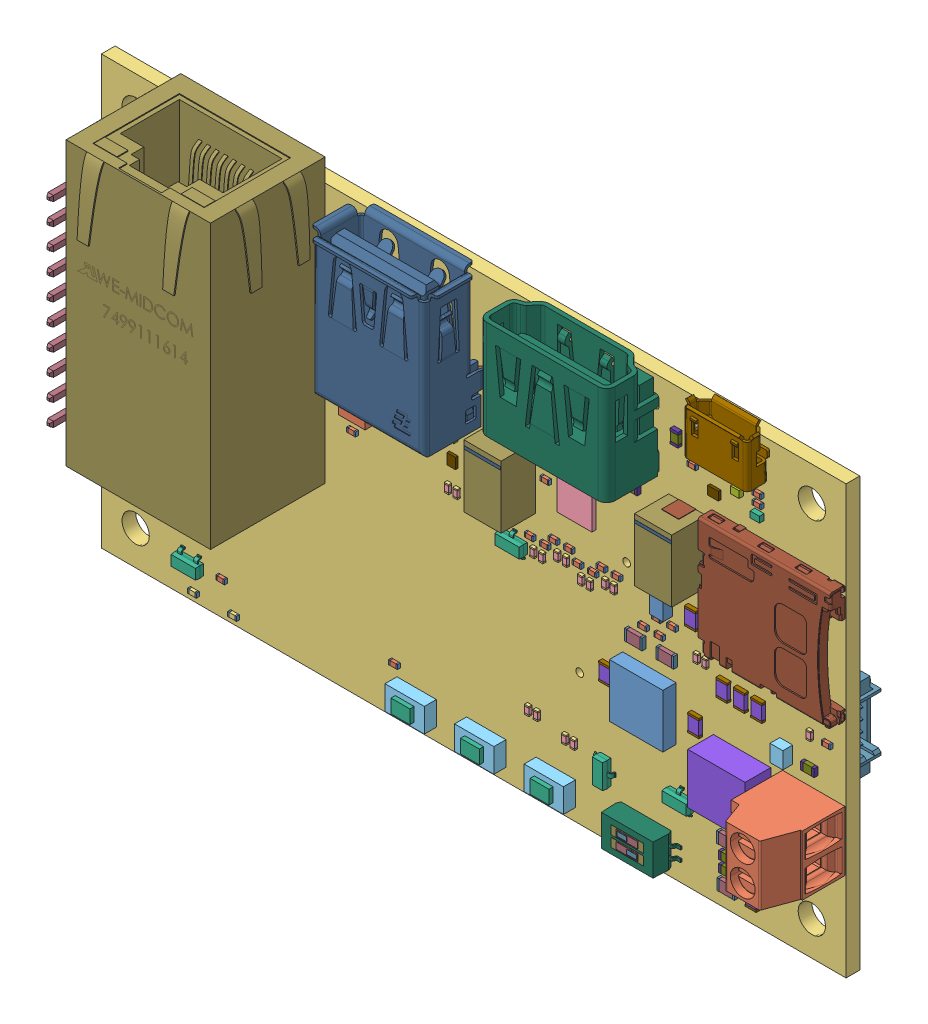
SolidWorks assembly ASG003_3D_MODEL, configuration Default. Lengths in mm.
Overall size (87.04 52.68 23.65).
962 component instances, 59 part files, 0 mates.
Components (placement in the parent):
- ASG003_3D_MODEL.step-1: ASG003_3D_MODEL.step [Default] at origin size (87.04 52.68 23.65)
  - R53.step-1: R53.step [Default] at origin size (1.02 0.52 0.36)
    - 870940480.step-1: 870940480.step [Default] at (7.8976 25.146 -1.9516) size (0.16 0.52 0.35)
      - Extruded.step-1: Extruded.step [Default] at origin size (0.16 0.52 0.35)
    - 870940480.step-2: 870940480.step [Default] at (7.0376 25.146 -1.9516) size (0.16 0.52 0.35)
      - Extruded.step-1: Extruded.step [Default] at origin size (0.16 0.52 0.35)
    - 870940640.step-1: 870940640.step [Default] at (7.4676 25.146 -1.9506) size (1.01 0.51 0.36)
      - Extruded-0.step-1: Extruded-0.step [Default] at origin size (1.01 0.51 0.36)
  - R52.step-1: R52.step [Default] at origin size (0.52 1.02 0.36)
    - 870941120.step-1: 870941120.step [Default] at (69.723 24.306 0) size (0.52 0.16 0.35)
      - Extruded-1.step-1: Extruded-1.step [Default] at origin size (0.52 0.16 0.35)
    - 870941120.step-2: 870941120.step [Default] at (69.723 23.446 0) size (0.52 0.16 0.35)
      - Extruded-1.step-1: Extruded-1.step [Default] at origin size (0.52 0.16 0.35)
    - 870941280.step-1: 870941280.step [Default] at (69.723 23.876 0) size (0.51 1.01 0.36)
      - Extruded-2.step-1: Extruded-2.step [Default] at origin size (0.51 1.01 0.36)
  - R40.step-1: R40.step [Default] at origin size (0.52 1.02 0.36)
    - 870941120.step-1: 870941120.step [Default] at (70.739 24.306 0) size (0.52 0.16 0.35)
      - Extruded-1.step-1: Extruded-1.step [Default] at origin size (0.52 0.16 0.35)
    - 870941120.step-2: 870941120.step [Default] at (70.739 23.446 0) size (0.52 0.16 0.35)
      - Extruded-1.step-1: Extruded-1.step [Default] at origin size (0.52 0.16 0.35)
    - 870941280.step-1: 870941280.step [Default] at (70.739 23.876 0) size (0.51 1.01 0.36)
      - Extruded-2.step-1: Extruded-2.step [Default] at origin size (0.51 1.01 0.36)
  - C59.step-1: C59.step [Default] at origin size (1.02 0.52 0.36)
    - 870940480.step-1: 870940480.step [Default] at (34.847 5.588 0) size (0.16 0.52 0.35)
      - Extruded.step-1: Extruded.step [Default] at origin size (0.16 0.52 0.35)
    - 870940480.step-2: 870940480.step [Default] at (33.987 5.588 0) size (0.16 0.52 0.35)
      - Extruded.step-1: Extruded.step [Default] at origin size (0.16 0.52 0.35)
    - 870940640.step-1: 870940640.step [Default] at (34.417 5.588 0) size (1.01 0.51 0.36)
      - Extruded-0.step-1: Extruded-0.step [Default] at origin size (1.01 0.51 0.36)
  - R51.step-1: R51.step [Default] at origin size (2.5 3.5 0.64)
    - 870944960.step-1: 870944960.step [Default] at (16.256 43.688 -2.2356) size (2.5 3.5 0.64)
      - Extruded-3.step-1: Extruded-3.step [Default] at origin size (2.5 3.5 0.64)
  - R14.step-1: R14.step [Default] at origin size (1.02 0.52 0.36)
    - 870940480.step-1: 870940480.step [Default] at (3.888 14.351 0) size (0.16 0.52 0.35)
      - Extruded.step-1: Extruded.step [Default] at origin size (0.16 0.52 0.35)
    - 870940480.step-2: 870940480.step [Default] at (4.748 14.351 0) size (0.16 0.52 0.35)
      - Extruded.step-1: Extruded.step [Default] at origin size (0.16 0.52 0.35)
    - 870940640.step-1: 870940640.step [Default] at (4.318 14.351 0) size (1.01 0.51 0.36)
      - Extruded-0.step-1: Extruded-0.step [Default] at origin size (1.01 0.51 0.36)
  - R13.step-1: R13.step [Default] at origin size (0.52 1.02 0.36)
    - 870941120.step-1: 870941120.step [Default] at (2.032 10.336 0) size (0.52 0.16 0.35)
      - Extruded-1.step-1: Extruded-1.step [Default] at origin size (0.52 0.16 0.35)
    - 870941120.step-2: 870941120.step [Default] at (2.032 9.476 0) size (0.52 0.16 0.35)
      - Extruded-1.step-1: Extruded-1.step [Default] at origin size (0.52 0.16 0.35)
    - 870941280.step-1: 870941280.step [Default] at (2.032 9.906 0) size (0.51 1.01 0.36)
      - Extruded-2.step-1: Extruded-2.step [Default] at origin size (0.51 1.01 0.36)
  - R12.step-1: R12.step [Default] at origin size (0.52 1.02 0.36)
    - 870941120.step-1: 870941120.step [Default] at (7.112 20.017 0) size (0.52 0.16 0.35)
      - Extruded-1.step-1: Extruded-1.step [Default] at origin size (0.52 0.16 0.35)
    - 870941120.step-2: 870941120.step [Default] at (7.112 20.877 0) size (0.52 0.16 0.35)
      - Extruded-1.step-1: Extruded-1.step [Default] at origin size (0.52 0.16 0.35)
    - 870941280.step-1: 870941280.step [Default] at (7.112 20.447 0) size (0.51 1.01 0.36)
      - Extruded-2.step-1: Extruded-2.step [Default] at origin size (0.51 1.01 0.36)
  - D1.step-1: D1.step [Default] at origin size (2.42 2.9 1)
    - SW3dPS-SOT-23.step-1: SW3dPS-SOT-23.step [Default] at (3.683 11.8109 0.498) x (1 0 0) z (0 -1 0) size (2.42 1 2.9)
  - C33.step-1: C33.step [Default] at origin size (2.72 3.52 2.51)
    - 870945120.step-1: 870945120.step [Default] at (19.431 43.688 -4.1006) size (2.7 3.5 2.5)
      - Extruded-4.step-1: Extruded-4.step [Default] at origin size (2.7 3.5 2.5)
    - 870945280.step-1: 870945280.step [Default] at (19.431 45.243 -4.1106) size (2.72 0.41 2.51)
      - Extruded-5.step-1: Extruded-5.step [Default] at origin size (2.72 0.41 2.51)
    - 870945280.step-2: 870945280.step [Default] at (19.431 42.133 -4.1106) size (2.72 0.41 2.51)
      - Extruded-5.step-1: Extruded-5.step [Default] at origin size (2.72 0.41 2.51)
  - C20.step-1: C20.step [Default] at origin size (1.02 0.52 0.36)
    - 870940480.step-1: 870940480.step [Default] at (3.634 9.271 0) size (0.16 0.52 0.35)
      - Extruded.step-1: Extruded.step [Default] at origin size (0.16 0.52 0.35)
    - 870940480.step-2: 870940480.step [Default] at (4.494 9.271 0) size (0.16 0.52 0.35)
      - Extruded.step-1: Extruded.step [Default] at origin size (0.16 0.52 0.35)
    - 870940640.step-1: 870940640.step [Default] at (4.064 9.271 0) size (1.01 0.51 0.36)
      - Extruded-0.step-1: Extruded-0.step [Default] at origin size (1.01 0.51 0.36)
  - C7.step-1: C7.step [Default] at origin size (1.02 0.52 0.36)
    - 870940480.step-1: 870940480.step [Default] at (13.794 4.064 0) size (0.16 0.52 0.35)
      - Extruded.step-1: Extruded.step [Default] at origin size (0.16 0.52 0.35)
    - 870940480.step-2: 870940480.step [Default] at (14.654 4.064 0) size (0.16 0.52 0.35)
      - Extruded.step-1: Extruded.step [Default] at origin size (0.16 0.52 0.35)
    - 870940640.step-1: 870940640.step [Default] at (14.224 4.064 0) size (1.01 0.51 0.36)
      - Extruded-0.step-1: Extruded-0.step [Default] at origin size (1.01 0.51 0.36)
  - U10.step-1: U10.step [Default] at origin size (1.26 2.01 0.91)
    - 870945920.step-1: 870945920.step [Default] at (16.6362 34.3856 -2.6006) size (1.26 2.01 0.91)
      - Extruded-6.step-1: Extruded-6.step [Default] at origin size (1.26 2.01 0.91)
  - U9.step-1: U9.step [Default] at origin size (2.9 1.75 0.99)
    - 870946400.step-1: 870946400.step [Default] at (19.9382 34.2586 -2.6006) size (2.9 1.75 0.99)
      - Extruded-7.step-1: Extruded-7.step [Default] at origin size (2.9 1.75 0.99)
  - U8.step-1: U8.step [Default] at origin size (1.26 2.01 0.91)
    - 870945920.step-1: 870945920.step [Default] at (17.6522 30.9566 -2.6006) size (1.26 2.01 0.91)
      - Extruded-6.step-1: Extruded-6.step [Default] at origin size (1.26 2.01 0.91)
  - U4.step-1: U4.step [Default] at origin size (3 1.7 1.45)
    - 870946240.step-1: 870946240.step [Default] at (13.3342 34.2586 -3.0506) size (3 1.7 1.45)
      - Extruded-8.step-1: Extruded-8.step [Default] at origin size (3 1.7 1.45)
  - S1.step-1: S1.step [Default] at origin size (8.13 3.66 2.38)
    - 870942400.step-1: 870942400.step [Default] at (63.7532 2.3346 1.27) size (3.81 1.02 1.07)
      - Extruded-9.step-1: Extruded-9.step [Default] at origin size (3.81 1.02 1.07)
    - 870942560.step-1: 870942560.step [Default] at (63.7532 2.3346 1.27) size (2.54 0.76 1.09)
      - Extruded-10.step-1: Extruded-10.step [Default] at origin size (2.54 0.76 1.09)
    - 870942720.step-1: 870942720.step [Default] at (64.3247 2.3346 1.27) size (1.14 0.51 1.12)
      - Extruded-11.step-1: Extruded-11.step [Default] at origin size (1.14 0.51 1.12)
    - 870942720.step-2: 870942720.step [Default] at (63.1817 3.6046 1.27) size (1.14 0.51 1.12)
      - Extruded-11.step-1: Extruded-11.step [Default] at origin size (1.14 0.51 1.12)
    - 870942560.step-2: 870942560.step [Default] at (63.7532 3.6046 1.27) size (2.54 0.76 1.09)
      - Extruded-10.step-1: Extruded-10.step [Default] at origin size (2.54 0.76 1.09)
    - 870942400.step-2: 870942400.step [Default] at (63.7532 3.6046 1.27) size (3.81 1.02 1.07)
      - Extruded-9.step-1: Extruded-9.step [Default] at origin size (3.81 1.02 1.07)
    - c-1571983-01-b-3d.step-1: c-1571983-01-b-3d.step [Default] at (63.7533 2.9696 0.571) x (0 1 0) z (0 0 1) size (3.66 8.13 2.31)
  - R50.step-1: R50.step [Default] at origin size (0.52 1.02 0.36)
    - 870941120.step-1: 870941120.step [Default] at (22.2242 30.5266 -1.9516) size (0.52 0.16 0.35)
      - Extruded-1.step-1: Extruded-1.step [Default] at origin size (0.52 0.16 0.35)
    - 870941120.step-2: 870941120.step [Default] at (22.2242 31.3866 -1.9516) size (0.52 0.16 0.35)
      - Extruded-1.step-1: Extruded-1.step [Default] at origin size (0.52 0.16 0.35)
    - 870941280.step-1: 870941280.step [Default] at (22.2242 30.9566 -1.9506) size (0.51 1.01 0.36)
      - Extruded-2.step-1: Extruded-2.step [Default] at origin size (0.51 1.01 0.36)
  - R49.step-1: R49.step [Default] at origin size (0.52 1.02 0.36)
    - 870941120.step-1: 870941120.step [Default] at (20.9542 37.8636 -1.9516) size (0.52 0.16 0.35)
      - Extruded-1.step-1: Extruded-1.step [Default] at origin size (0.52 0.16 0.35)
    - 870941120.step-2: 870941120.step [Default] at (20.9542 37.0036 -1.9516) size (0.52 0.16 0.35)
      - Extruded-1.step-1: Extruded-1.step [Default] at origin size (0.52 0.16 0.35)
    - 870941280.step-1: 870941280.step [Default] at (20.9542 37.4336 -1.9506) size (0.51 1.01 0.36)
      - Extruded-2.step-1: Extruded-2.step [Default] at origin size (0.51 1.01 0.36)
  - R48.step-1: R48.step [Default] at origin size (0.52 1.02 0.36)
    - 870941120.step-1: 870941120.step [Default] at (21.0812 31.3866 -1.9516) size (0.52 0.16 0.35)
      - Extruded-1.step-1: Extruded-1.step [Default] at origin size (0.52 0.16 0.35)
    - 870941120.step-2: 870941120.step [Default] at (21.0812 30.5266 -1.9516) size (0.52 0.16 0.35)
      - Extruded-1.step-1: Extruded-1.step [Default] at origin size (0.52 0.16 0.35)
    - 870941280.step-1: 870941280.step [Default] at (21.0812 30.9566 -1.9506) size (0.51 1.01 0.36)
      - Extruded-2.step-1: Extruded-2.step [Default] at origin size (0.51 1.01 0.36)
  - R22.step-1: R22.step [Default] at origin size (0.52 1.02 0.36)
    - 870941120.step-1: 870941120.step [Default] at (15.3662 32.0216 -1.9516) size (0.52 0.16 0.35)
      - Extruded-1.step-1: Extruded-1.step [Default] at origin size (0.52 0.16 0.35)
    - 870941120.step-2: 870941120.step [Default] at (15.3662 31.1616 -1.9516) size (0.52 0.16 0.35)
      - Extruded-1.step-1: Extruded-1.step [Default] at origin size (0.52 0.16 0.35)
    - 870941280.step-1: 870941280.step [Default] at (15.3662 31.5916 -1.9506) size (0.51 1.01 0.36)
      - Extruded-2.step-1: Extruded-2.step [Default] at origin size (0.51 1.01 0.36)
  - R18.step-1: R18.step [Default] at origin size (0.52 1.02 0.36)
    - 870941120.step-1: 870941120.step [Default] at (78.867 21.795 -1.9516) size (0.52 0.16 0.35)
      - Extruded-1.step-1: Extruded-1.step [Default] at origin size (0.52 0.16 0.35)
    - 870941120.step-2: 870941120.step [Default] at (78.867 22.655 -1.9516) size (0.52 0.16 0.35)
      - Extruded-1.step-1: Extruded-1.step [Default] at origin size (0.52 0.16 0.35)
    - 870941280.step-1: 870941280.step [Default] at (78.867 22.225 -1.9506) size (0.51 1.01 0.36)
      - Extruded-2.step-1: Extruded-2.step [Default] at origin size (0.51 1.01 0.36)
  - L7.step-1: L7.step [Default] at origin size (1.6 0.9 0.46)
    - 870942240.step-1: 870942240.step [Default] at (75.692 25.273 -2.0506) size (1 0.9 0.45)
      - Extruded-12.step-1: Extruded-12.step [Default] at origin size (1 0.9 0.45)
    - 870942080.step-1: 870942080.step [Default] at (76.342 25.273 -2.0606) size (0.3 0.9 0.46)
      - Extruded-13.step-1: Extruded-13.step [Default] at origin size (0.3 0.9 0.46)
    - 870942080.step-2: 870942080.step [Default] at (75.042 25.273 -2.0606) size (0.3 0.9 0.46)
      - Extruded-13.step-1: Extruded-13.step [Default] at origin size (0.3 0.9 0.46)
  - C58.step-1: C58.step [Default] at origin size (0.52 1.02 0.36)
    - 870941120.step-1: 870941120.step [Default] at (19.9382 31.3866 -1.9516) size (0.52 0.16 0.35)
      - Extruded-1.step-1: Extruded-1.step [Default] at origin size (0.52 0.16 0.35)
    - 870941120.step-2: 870941120.step [Default] at (19.9382 30.5266 -1.9516) size (0.52 0.16 0.35)
      - Extruded-1.step-1: Extruded-1.step [Default] at origin size (0.52 0.16 0.35)
    - 870941280.step-1: 870941280.step [Default] at (19.9382 30.9566 -1.9506) size (0.51 1.01 0.36)
      - Extruded-2.step-1: Extruded-2.step [Default] at origin size (0.51 1.01 0.36)
  - C50.step-1: C50.step [Default] at origin size (0.52 1.02 0.36)
    - 870941120.step-1: 870941120.step [Default] at (12.4452 36.7496 -1.9516) size (0.52 0.16 0.35)
      - Extruded-1.step-1: Extruded-1.step [Default] at origin size (0.52 0.16 0.35)
    - 870941120.step-2: 870941120.step [Default] at (12.4452 37.6096 -1.9516) size (0.52 0.16 0.35)
      - Extruded-1.step-1: Extruded-1.step [Default] at origin size (0.52 0.16 0.35)
    - 870941280.step-1: 870941280.step [Default] at (12.4452 37.1796 -1.9506) size (0.51 1.01 0.36)
      - Extruded-2.step-1: Extruded-2.step [Default] at origin size (0.51 1.01 0.36)
  - C49.step-1: C49.step [Default] at origin size (0.52 1.02 0.36)
    - 870941120.step-1: 870941120.step [Default] at (14.3502 36.8076 -1.9516) size (0.52 0.16 0.35)
      - Extruded-1.step-1: Extruded-1.step [Default] at origin size (0.52 0.16 0.35)
    - 870941120.step-2: 870941120.step [Default] at (14.3502 37.6676 -1.9516) size (0.52 0.16 0.35)
      - Extruded-1.step-1: Extruded-1.step [Default] at origin size (0.52 0.16 0.35)
    - 870941280.step-1: 870941280.step [Default] at (14.3502 37.2376 -1.9506) size (0.51 1.01 0.36)
      - Extruded-2.step-1: Extruded-2.step [Default] at origin size (0.51 1.01 0.36)
  - C48.step-1: C48.step [Default] at origin size (1.02 0.52 0.36)
    - 870940480.step-1: 870940480.step [Default] at (84.533 22.733 0) size (0.16 0.52 0.35)
      - Extruded.step-1: Extruded.step [Default] at origin size (0.16 0.52 0.35)
    - 870940480.step-2: 870940480.step [Default] at (85.393 22.733 0) size (0.16 0.52 0.35)
      - Extruded.step-1: Extruded.step [Default] at origin size (0.16 0.52 0.35)
    - 870940640.step-1: 870940640.step [Default] at (84.963 22.733 0) size (1.01 0.51 0.36)
      - Extruded-0.step-1: Extruded-0.step [Default] at origin size (1.01 0.51 0.36)
  - R47.step-1: R47.step [Default] at origin size (1.02 0.52 0.36)
    - 870940480.step-1: 870940480.step [Default] at (63.9292 23.9246 0) size (0.16 0.52 0.35)
      - Extruded.step-1: Extruded.step [Default] at origin size (0.16 0.52 0.35)
    - 870940480.step-2: 870940480.step [Default] at (63.0692 23.9246 0) size (0.16 0.52 0.35)
      - Extruded.step-1: Extruded.step [Default] at origin size (0.16 0.52 0.35)
    - 870940640.step-1: 870940640.step [Default] at (63.4992 23.9246 0) size (1.01 0.51 0.36)
      - Extruded-0.step-1: Extruded-0.step [Default] at origin size (1.01 0.51 0.36)
  - R46.step-1: R46.step [Default] at origin size (0.52 1.02 0.36)
    - 870941120.step-1: 870941120.step [Default] at (8.255 20.017 0) size (0.52 0.16 0.35)
      - Extruded-1.step-1: Extruded-1.step [Default] at origin size (0.52 0.16 0.35)
    - 870941120.step-2: 870941120.step [Default] at (8.255 20.877 0) size (0.52 0.16 0.35)
      - Extruded-1.step-1: Extruded-1.step [Default] at origin size (0.52 0.16 0.35)
    - 870941280.step-1: 870941280.step [Default] at (8.255 20.447 0) size (0.51 1.01 0.36)
      - Extruded-2.step-1: Extruded-2.step [Default] at origin size (0.51 1.01 0.36)
  - L1.step-1: L1.step [Default] at origin size (1 1.25 0.29)
    - 870940800.step-1: 870940800.step [Default] at (44.881 29.538 0.005) size (1 1.25 0.29)
      - Extruded-14.step-1: Extruded-14.step [Default] at origin size (1 1.25 0.29)
  - U7.step-1: U7.step [Default] at origin size (1.6 3 1.1)
    - 870944800.step-1: 870944800.step [Default] at (65.913 27.94 0) size (1.6 3 1.1)
      - Extruded-15.step-1: Extruded-15.step [Default] at origin size (1.6 3 1.1)
  - U5.step-1: U5.step [Default] at origin size (3.1 3.1 0.95)
    - 870940320.step-1: 870940320.step [Default] at (30.2506 29.8936 0.05) size (3.1 3.1 0.95)
      - Extruded-16.step-1: Extruded-16.step [Default] at origin size (3.1 3.1 0.95)
  - U3.step-1: U3.step [Default] at origin size (3.65 3.65 0.95)
    - 870946080.step-1: 870946080.step [Default] at (8.751 30.152 -2.6006) size (3.65 3.65 0.95)
      - Extruded-17.step-1: Extruded-17.step [Default] at origin size (3.65 3.65 0.95)
  - U2.step-1: U2.step [Default] at origin size (3.65 3.65 0.95)
    - 870946080.step-1: 870946080.step [Default] at (8.751 37.539 -2.6006) size (3.65 3.65 0.95)
      - Extruded-17.step-1: Extruded-17.step [Default] at origin size (3.65 3.65 0.95)
  - U1.step-1: U1.step [Default] at origin size (4.1 4.1 0.5)
    - 870941920.step-1: 870941920.step [Default] at (55.7522 32.8146 0) size (4.1 4.1 0.5)
      - Extruded-18.step-1: Extruded-18.step [Default] at origin size (4.1 4.1 0.5)
  - SW3.step-1: SW3.step [Default] at origin size (4.6 2.8 1.9)
    - 870942880.step-1: 870942880.step [Default] at (44.9573 2.8427 0) size (4.6 2.8 1.4)
      - Extruded-19.step-1: Extruded-19.step [Default] at origin size (4.6 2.8 1.4)
    - 870943040.step-1: 870943040.step [Default] at (44.9572 2.8426 1.4) size (2.2 1.6 0.5)
      - Extruded-20.step-1: Extruded-20.step [Default] at origin size (2.2 1.6 0.5)
  - SW2.step-1: SW2.step [Default] at origin size (4.6 2.8 1.9)
    - 870942880.step-1: 870942880.step [Default] at (53.0853 2.8427 0) size (4.6 2.8 1.4)
      - Extruded-19.step-1: Extruded-19.step [Default] at origin size (4.6 2.8 1.4)
    - 870943040.step-1: 870943040.step [Default] at (53.0852 2.8426 1.4) size (2.2 1.6 0.5)
      - Extruded-20.step-1: Extruded-20.step [Default] at origin size (2.2 1.6 0.5)
  - SW1.step-1: SW1.step [Default] at origin size (4.6 2.8 1.9)
    - 870942880.step-1: 870942880.step [Default] at (36.8293 2.8427 0) size (4.6 2.8 1.4)
      - Extruded-19.step-1: Extruded-19.step [Default] at origin size (4.6 2.8 1.4)
    - 870943040.step-1: 870943040.step [Default] at (36.8292 2.8426 1.4) size (2.2 1.6 0.5)
      - Extruded-20.step-1: Extruded-20.step [Default] at origin size (2.2 1.6 0.5)
  - R45.step-1: R45.step [Default] at origin size (1.02 0.52 0.36)
    - 870940480.step-1: 870940480.step [Default] at (64.6964 25.5915 0) size (0.16 0.52 0.35)
      - Extruded.step-1: Extruded.step [Default] at origin size (0.16 0.52 0.35)
    - 870940480.step-2: 870940480.step [Default] at (65.5564 25.5915 0) size (0.16 0.52 0.35)
      - Extruded.step-1: Extruded.step [Default] at origin size (0.16 0.52 0.35)
    - 870940640.step-1: 870940640.step [Default] at (65.1264 25.5915 0) size (1.01 0.51 0.36)
      - Extruded-0.step-1: Extruded-0.step [Default] at origin size (1.01 0.51 0.36)
  - R44.step-1: R44.step [Default] at origin size (1.02 0.52 0.36)
    - 870940480.step-1: 870940480.step [Default] at (66.4744 25.5915 0) size (0.16 0.52 0.35)
      - Extruded.step-1: Extruded.step [Default] at origin size (0.16 0.52 0.35)
    - 870940480.step-2: 870940480.step [Default] at (67.3344 25.5915 0) size (0.16 0.52 0.35)
      - Extruded.step-1: Extruded.step [Default] at origin size (0.16 0.52 0.35)
    - 870940640.step-1: 870940640.step [Default] at (66.9044 25.5915 0) size (1.01 0.51 0.36)
      - Extruded-0.step-1: Extruded-0.step [Default] at origin size (1.01 0.51 0.36)
  - R39.step-1: R39.step [Default] at origin size (1.6 0.9 0.46)
    - 870942080.step-1: 870942080.step [Default] at (83.581 19.304 0) size (0.3 0.9 0.46)
      - Extruded-13.step-1: Extruded-13.step [Default] at origin size (0.3 0.9 0.46)
    - 870942080.step-2: 870942080.step [Default] at (82.281 19.304 0) size (0.3 0.9 0.46)
      - Extruded-13.step-1: Extruded-13.step [Default] at origin size (0.3 0.9 0.46)
    - 870942240.step-1: 870942240.step [Default] at (82.931 19.304 0) size (1 0.9 0.45)
      - Extruded-12.step-1: Extruded-12.step [Default] at origin size (1 0.9 0.45)
  - R38.step-1: R38.step [Default] at origin size (1.02 0.52 0.36)
    - 870940480.step-1: 870940480.step [Default] at (67.3872 19.3526 -1.9516) size (0.16 0.52 0.35)
      - Extruded.step-1: Extruded.step [Default] at origin size (0.16 0.52 0.35)
    - 870940480.step-2: 870940480.step [Default] at (68.2472 19.3526 -1.9516) size (0.16 0.52 0.35)
      - Extruded.step-1: Extruded.step [Default] at origin size (0.16 0.52 0.35)
    - 870940640.step-1: 870940640.step [Default] at (67.8172 19.3526 -1.9506) size (1.01 0.51 0.36)
      - Extruded-0.step-1: Extruded-0.step [Default] at origin size (1.01 0.51 0.36)
  - R37.step-1: R37.step [Default] at origin size (1.02 0.52 0.36)
    - 870940480.step-1: 870940480.step [Default] at (61.3892 19.3526 -1.9516) size (0.16 0.52 0.35)
      - Extruded.step-1: Extruded.step [Default] at origin size (0.16 0.52 0.35)
    - 870940480.step-2: 870940480.step [Default] at (60.5292 19.3526 -1.9516) size (0.16 0.52 0.35)
      - Extruded.step-1: Extruded.step [Default] at origin size (0.16 0.52 0.35)
    - 870940640.step-1: 870940640.step [Default] at (60.9592 19.3526 -1.9506) size (1.01 0.51 0.36)
      - Extruded-0.step-1: Extruded-0.step [Default] at origin size (1.01 0.51 0.36)
  - R36.step-1: R36.step [Default] at origin size (1.02 0.52 0.36)
    - 870940480.step-1: 870940480.step [Default] at (64.9742 23.9246 0) size (0.16 0.52 0.35)
      - Extruded.step-1: Extruded.step [Default] at origin size (0.16 0.52 0.35)
    - 870940480.step-2: 870940480.step [Default] at (65.8342 23.9246 0) size (0.16 0.52 0.35)
      - Extruded.step-1: Extruded.step [Default] at origin size (0.16 0.52 0.35)
    - 870940640.step-1: 870940640.step [Default] at (65.4042 23.9246 0) size (1.01 0.51 0.36)
      - Extruded-0.step-1: Extruded-0.step [Default] at origin size (1.01 0.51 0.36)
  - R35.step-1: R35.step [Default] at origin size (0.52 1.02 0.36)
    - 870941120.step-1: 870941120.step [Default] at (32.0286 29.6596 -1.9516) size (0.52 0.16 0.35)
      - Extruded-1.step-1: Extruded-1.step [Default] at origin size (0.52 0.16 0.35)
    - 870941120.step-2: 870941120.step [Default] at (32.0286 30.5196 -1.9516) size (0.52 0.16 0.35)
      - Extruded-1.step-1: Extruded-1.step [Default] at origin size (0.52 0.16 0.35)
    - 870941280.step-1: 870941280.step [Default] at (32.0286 30.0896 -1.9506) size (0.51 1.01 0.36)
      - Extruded-2.step-1: Extruded-2.step [Default] at origin size (0.51 1.01 0.36)
  - R34.step-1: R34.step [Default] at origin size (1.02 0.52 0.36)
    - 870940480.step-1: 870940480.step [Default] at (32.865 28.6744 -1.9516) size (0.16 0.52 0.35)
      - Extruded.step-1: Extruded.step [Default] at origin size (0.16 0.52 0.35)
    - 870940480.step-2: 870940480.step [Default] at (32.005 28.6744 -1.9516) size (0.16 0.52 0.35)
      - Extruded.step-1: Extruded.step [Default] at origin size (0.16 0.52 0.35)
    - 870940640.step-1: 870940640.step [Default] at (32.435 28.6744 -1.9506) size (1.01 0.51 0.36)
      - Extruded-0.step-1: Extruded-0.step [Default] at origin size (1.01 0.51 0.36)
  - R33.step-1: R33.step [Default] at origin size (1.02 0.52 0.36)
    - 870940480.step-1: 870940480.step [Default] at (69.695 43.127 0) size (0.16 0.52 0.35)
      - Extruded.step-1: Extruded.step [Default] at origin size (0.16 0.52 0.35)
    - 870940480.step-2: 870940480.step [Default] at (68.835 43.127 0) size (0.16 0.52 0.35)
      - Extruded.step-1: Extruded.step [Default] at origin size (0.16 0.52 0.35)
    - 870940640.step-1: 870940640.step [Default] at (69.265 43.127 0) size (1.01 0.51 0.36)
      - Extruded-0.step-1: Extruded-0.step [Default] at origin size (1.01 0.51 0.36)
  - R32.step-1: R32.step [Default] at origin size (1.02 0.52 0.36)
    - 870940480.step-1: 870940480.step [Default] at (30.6806 31.2906 -1.9516) size (0.16 0.52 0.35)
      - Extruded.step-1: Extruded.step [Default] at origin size (0.16 0.52 0.35)
    - 870940480.step-2: 870940480.step [Default] at (29.8206 31.2906 -1.9516) size (0.16 0.52 0.35)
      - Extruded.step-1: Extruded.step [Default] at origin size (0.16 0.52 0.35)
    - 870940640.step-1: 870940640.step [Default] at (30.2506 31.2906 -1.9506) size (1.01 0.51 0.36)
      - Extruded-0.step-1: Extruded-0.step [Default] at origin size (1.01 0.51 0.36)
  - R31.step-1: R31.step [Default] at origin size (0.52 1.02 0.36)
    - 870941120.step-1: 870941120.step [Default] at (28.4726 29.7176 -1.9516) size (0.52 0.16 0.35)
      - Extruded-1.step-1: Extruded-1.step [Default] at origin size (0.52 0.16 0.35)
    - 870941120.step-2: 870941120.step [Default] at (28.4726 30.5776 -1.9516) size (0.52 0.16 0.35)
      - Extruded-1.step-1: Extruded-1.step [Default] at origin size (0.52 0.16 0.35)
    - 870941280.step-1: 870941280.step [Default] at (28.4726 30.1476 -1.9506) size (0.51 1.01 0.36)
      - Extruded-2.step-1: Extruded-2.step [Default] at origin size (0.51 1.01 0.36)
  - R30.step-1: R30.step [Default] at origin size (1.02 0.52 0.36)
    - 870940480.step-1: 870940480.step [Default] at (27.6362 28.6998 -1.9516) size (0.16 0.52 0.35)
      - Extruded.step-1: Extruded.step [Default] at origin size (0.16 0.52 0.35)
    - 870940480.step-2: 870940480.step [Default] at (28.4962 28.6998 -1.9516) size (0.16 0.52 0.35)
      - Extruded.step-1: Extruded.step [Default] at origin size (0.16 0.52 0.35)
    - 870940640.step-1: 870940640.step [Default] at (28.0662 28.6998 -1.9506) size (1.01 0.51 0.36)
      - Extruded-0.step-1: Extruded-0.step [Default] at origin size (1.01 0.51 0.36)
  - R29.step-1: R29.step [Default] at origin size (0.52 1.02 0.36)
    - 870941120.step-1: 870941120.step [Default] at (68.884 46.224 0) size (0.52 0.16 0.35)
      - Extruded-1.step-1: Extruded-1.step [Default] at origin size (0.52 0.16 0.35)
    - 870941120.step-2: 870941120.step [Default] at (68.884 45.364 0) size (0.52 0.16 0.35)
      - Extruded-1.step-1: Extruded-1.step [Default] at origin size (0.52 0.16 0.35)
    - 870941280.step-1: 870941280.step [Default] at (68.884 45.794 0) size (0.51 1.01 0.36)
      - Extruded-2.step-1: Extruded-2.step [Default] at origin size (0.51 1.01 0.36)
  - R28.step-1: R28.step [Default] at origin size (0.52 1.02 0.36)
    - 870941120.step-1: 870941120.step [Default] at (51.054 8.333 0) size (0.52 0.16 0.35)
      - Extruded-1.step-1: Extruded-1.step [Default] at origin size (0.52 0.16 0.35)
    - 870941120.step-2: 870941120.step [Default] at (51.054 9.193 0) size (0.52 0.16 0.35)
      - Extruded-1.step-1: Extruded-1.step [Default] at origin size (0.52 0.16 0.35)
    - 870941280.step-1: 870941280.step [Default] at (51.054 8.763 0) size (0.51 1.01 0.36)
      - Extruded-2.step-1: Extruded-2.step [Default] at origin size (0.51 1.01 0.36)
  - R27.step-1: R27.step [Default] at origin size (0.52 1.02 0.36)
    - 870941120.step-1: 870941120.step [Default] at (50.038 9.193 0) size (0.52 0.16 0.35)
      - Extruded-1.step-1: Extruded-1.step [Default] at origin size (0.52 0.16 0.35)
    - 870941120.step-2: 870941120.step [Default] at (50.038 8.333 0) size (0.52 0.16 0.35)
      - Extruded-1.step-1: Extruded-1.step [Default] at origin size (0.52 0.16 0.35)
    - 870941280.step-1: 870941280.step [Default] at (50.038 8.763 0) size (0.51 1.01 0.36)
      - Extruded-2.step-1: Extruded-2.step [Default] at origin size (0.51 1.01 0.36)
  - R26.step-1: R26.step [Default] at origin size (0.52 1.02 0.36)
    - 870941120.step-1: 870941120.step [Default] at (73.66 34.466 -1.9516) size (0.52 0.16 0.35)
      - Extruded-1.step-1: Extruded-1.step [Default] at origin size (0.52 0.16 0.35)
    - 870941120.step-2: 870941120.step [Default] at (73.66 33.606 -1.9516) size (0.52 0.16 0.35)
      - Extruded-1.step-1: Extruded-1.step [Default] at origin size (0.52 0.16 0.35)
    - 870941280.step-1: 870941280.step [Default] at (73.66 34.036 -1.9506) size (0.51 1.01 0.36)
      - Extruded-2.step-1: Extruded-2.step [Default] at origin size (0.51 1.01 0.36)
  - R25.step-1: R25.step [Default] at origin size (1.02 0.52 0.36)
    - 870940480.step-1: 870940480.step [Default] at (78.183 29.337 -1.9516) size (0.16 0.52 0.35)
      - Extruded.step-1: Extruded.step [Default] at origin size (0.16 0.52 0.35)
    - 870940480.step-2: 870940480.step [Default] at (79.043 29.337 -1.9516) size (0.16 0.52 0.35)
      - Extruded.step-1: Extruded.step [Default] at origin size (0.16 0.52 0.35)
    - 870940640.step-1: 870940640.step [Default] at (78.613 29.337 -1.9506) size (1.01 0.51 0.36)
      - Extruded-0.step-1: Extruded-0.step [Default] at origin size (1.01 0.51 0.36)
  - R24.step-1: R24.step [Default] at origin size (0.52 1.02 0.36)
    - 870941120.step-1: 870941120.step [Default] at (20.878 18.694 -1.9516) size (0.52 0.16 0.35)
      - Extruded-1.step-1: Extruded-1.step [Default] at origin size (0.52 0.16 0.35)
    - 870941120.step-2: 870941120.step [Default] at (20.878 19.554 -1.9516) size (0.52 0.16 0.35)
      - Extruded-1.step-1: Extruded-1.step [Default] at origin size (0.52 0.16 0.35)
    - 870941280.step-1: 870941280.step [Default] at (20.878 19.124 -1.9506) size (0.51 1.01 0.36)
      - Extruded-2.step-1: Extruded-2.step [Default] at origin size (0.51 1.01 0.36)
  - R23.step-1: R23.step [Default] at origin size (0.52 1.02 0.36)
    - 870941120.step-1: 870941120.step [Default] at (10.464 18.694 -1.9516) size (0.52 0.16 0.35)
      - Extruded-1.step-1: Extruded-1.step [Default] at origin size (0.52 0.16 0.35)
    - 870941120.step-2: 870941120.step [Default] at (10.464 19.554 -1.9516) size (0.52 0.16 0.35)
      - Extruded-1.step-1: Extruded-1.step [Default] at origin size (0.52 0.16 0.35)
    - 870941280.step-1: 870941280.step [Default] at (10.464 19.124 -1.9506) size (0.51 1.01 0.36)
      - Extruded-2.step-1: Extruded-2.step [Default] at origin size (0.51 1.01 0.36)
  - R20.step-1: R20.step [Default] at origin size (1.02 0.52 0.36)
    - 870940480.step-1: 870940480.step [Default] at (7.854 26.67 -1.9516) size (0.16 0.52 0.35)
      - Extruded.step-1: Extruded.step [Default] at origin size (0.16 0.52 0.35)
    - 870940480.step-2: 870940480.step [Default] at (6.994 26.67 -1.9516) size (0.16 0.52 0.35)
      - Extruded.step-1: Extruded.step [Default] at origin size (0.16 0.52 0.35)
    - 870940640.step-1: 870940640.step [Default] at (7.424 26.67 -1.9506) size (1.01 0.51 0.36)
      - Extruded-0.step-1: Extruded-0.step [Default] at origin size (1.01 0.51 0.36)
  - R21.step-1: R21.step [Default] at origin size (1.02 0.52 0.36)
    - 870940480.step-1: 870940480.step [Default] at (18.8442 37.0526 -1.9516) size (0.16 0.52 0.35)
      - Extruded.step-1: Extruded.step [Default] at origin size (0.16 0.52 0.35)
    - 870940480.step-2: 870940480.step [Default] at (17.9842 37.0526 -1.9516) size (0.16 0.52 0.35)
      - Extruded.step-1: Extruded.step [Default] at origin size (0.16 0.52 0.35)
    - 870940640.step-1: 870940640.step [Default] at (18.4142 37.0526 -1.9506) size (1.01 0.51 0.36)
      - Extruded-0.step-1: Extruded-0.step [Default] at origin size (1.01 0.51 0.36)
  - R19.step-1: R19.step [Default] at origin size (0.52 1.02 0.36)
    - 870941120.step-1: 870941120.step [Default] at (55.372 8.431 0) size (0.52 0.16 0.35)
      - Extruded-1.step-1: Extruded-1.step [Default] at origin size (0.52 0.16 0.35)
    - 870941120.step-2: 870941120.step [Default] at (55.372 7.571 0) size (0.52 0.16 0.35)
      - Extruded-1.step-1: Extruded-1.step [Default] at origin size (0.52 0.16 0.35)
    - 870941280.step-1: 870941280.step [Default] at (55.372 8.001 0) size (0.51 1.01 0.36)
      - Extruded-2.step-1: Extruded-2.step [Default] at origin size (0.51 1.01 0.36)
  - R15.step-1: R15.step [Default] at origin size (1.02 0.52 0.36)
    - 870940480.step-1: 870940480.step [Default] at (7.923 34.671 -1.9516) size (0.16 0.52 0.35)
      - Extruded.step-1: Extruded.step [Default] at origin size (0.16 0.52 0.35)
    - 870940480.step-2: 870940480.step [Default] at (7.063 34.671 -1.9516) size (0.16 0.52 0.35)
      - Extruded.step-1: Extruded.step [Default] at origin size (0.16 0.52 0.35)
    - 870940640.step-1: 870940640.step [Default] at (7.493 34.671 -1.9506) size (1.01 0.51 0.36)
      - Extruded-0.step-1: Extruded-0.step [Default] at origin size (1.01 0.51 0.36)
  - R17.step-1: R17.step [Default] at origin size (0.52 1.02 0.36)
    - 870941120.step-1: 870941120.step [Default] at (54.356 7.571 0) size (0.52 0.16 0.35)
      - Extruded-1.step-1: Extruded-1.step [Default] at origin size (0.52 0.16 0.35)
    - 870941120.step-2: 870941120.step [Default] at (54.356 8.431 0) size (0.52 0.16 0.35)
      - Extruded-1.step-1: Extruded-1.step [Default] at origin size (0.52 0.16 0.35)
    - 870941280.step-1: 870941280.step [Default] at (54.356 8.001 0) size (0.51 1.01 0.36)
      - Extruded-2.step-1: Extruded-2.step [Default] at origin size (0.51 1.01 0.36)
  - R16.step-1: R16.step [Default] at origin size (0.52 1.02 0.36)
    - 870941120.step-1: 870941120.step [Default] at (82.931 22.245 0) size (0.52 0.16 0.35)
      - Extruded-1.step-1: Extruded-1.step [Default] at origin size (0.52 0.16 0.35)
    - 870941120.step-2: 870941120.step [Default] at (82.931 23.105 0) size (0.52 0.16 0.35)
      - Extruded-1.step-1: Extruded-1.step [Default] at origin size (0.52 0.16 0.35)
    - 870941280.step-1: 870941280.step [Default] at (82.931 22.675 0) size (0.51 1.01 0.36)
      - Extruded-2.step-1: Extruded-2.step [Default] at origin size (0.51 1.01 0.36)
  - R11.step-1: R11.step [Default] at origin size (1.02 0.52 0.36)
    - 870940480.step-1: 870940480.step [Default] at (52.4738 26.4392 0) size (0.16 0.52 0.35)
      - Extruded.step-1: Extruded.step [Default] at origin size (0.16 0.52 0.35)
    - 870940480.step-2: 870940480.step [Default] at (51.6138 26.4392 0) size (0.16 0.52 0.35)
      - Extruded.step-1: Extruded.step [Default] at origin size (0.16 0.52 0.35)
    - 870940640.step-1: 870940640.step [Default] at (52.0438 26.4392 0) size (1.01 0.51 0.36)
      - Extruded-0.step-1: Extruded-0.step [Default] at origin size (1.01 0.51 0.36)
  - R10.step-1: R10.step [Default] at origin size (1.02 0.52 0.36)
    - 870940480.step-1: 870940480.step [Default] at (49.8358 26.4392 0) size (0.16 0.52 0.35)
      - Extruded.step-1: Extruded.step [Default] at origin size (0.16 0.52 0.35)
    - 870940480.step-2: 870940480.step [Default] at (50.6958 26.4392 0) size (0.16 0.52 0.35)
      - Extruded.step-1: Extruded.step [Default] at origin size (0.16 0.52 0.35)
    - 870940640.step-1: 870940640.step [Default] at (50.2658 26.4392 0) size (1.01 0.51 0.36)
      - Extruded-0.step-1: Extruded-0.step [Default] at origin size (1.01 0.51 0.36)
  - R9.step-1: R9.step [Default] at origin size (1.02 0.52 0.36)
    - 870940480.step-1: 870940480.step [Default] at (55.2678 27.4552 0) size (0.16 0.52 0.35)
      - Extruded.step-1: Extruded.step [Default] at origin size (0.16 0.52 0.35)
    - 870940480.step-2: 870940480.step [Default] at (54.4078 27.4552 0) size (0.16 0.52 0.35)
      - Extruded.step-1: Extruded.step [Default] at origin size (0.16 0.52 0.35)
    - 870940640.step-1: 870940640.step [Default] at (54.8378 27.4552 0) size (1.01 0.51 0.36)
      - Extruded-0.step-1: Extruded-0.step [Default] at origin size (1.01 0.51 0.36)
  - R8.step-1: R8.step [Default] at origin size (1.02 0.52 0.36)
    - 870940480.step-1: 870940480.step [Default] at (52.6298 27.4552 0) size (0.16 0.52 0.35)
      - Extruded.step-1: Extruded.step [Default] at origin size (0.16 0.52 0.35)
    - 870940480.step-2: 870940480.step [Default] at (53.4898 27.4552 0) size (0.16 0.52 0.35)
      - Extruded.step-1: Extruded.step [Default] at origin size (0.16 0.52 0.35)
    - 870940640.step-1: 870940640.step [Default] at (53.0598 27.4552 0) size (1.01 0.51 0.36)
      - Extruded-0.step-1: Extruded-0.step [Default] at origin size (1.01 0.51 0.36)
  - R7.step-1: R7.step [Default] at origin size (1.02 0.52 0.36)
    - 870940480.step-1: 870940480.step [Default] at (58.0618 26.4392 0) size (0.16 0.52 0.35)
      - Extruded.step-1: Extruded.step [Default] at origin size (0.16 0.52 0.35)
    - 870940480.step-2: 870940480.step [Default] at (57.2018 26.4392 0) size (0.16 0.52 0.35)
      - Extruded.step-1: Extruded.step [Default] at origin size (0.16 0.52 0.35)
    - 870940640.step-1: 870940640.step [Default] at (57.6318 26.4392 0) size (1.01 0.51 0.36)
      - Extruded-0.step-1: Extruded-0.step [Default] at origin size (1.01 0.51 0.36)
  - R6.step-1: R6.step [Default] at origin size (1.02 0.52 0.36)
    - 870940480.step-1: 870940480.step [Default] at (55.4238 26.4392 0) size (0.16 0.52 0.35)
      - Extruded.step-1: Extruded.step [Default] at origin size (0.16 0.52 0.35)
    - 870940480.step-2: 870940480.step [Default] at (56.2838 26.4392 0) size (0.16 0.52 0.35)
      - Extruded.step-1: Extruded.step [Default] at origin size (0.16 0.52 0.35)
    - 870940640.step-1: 870940640.step [Default] at (55.8538 26.4392 0) size (1.01 0.51 0.36)
      - Extruded-0.step-1: Extruded-0.step [Default] at origin size (1.01 0.51 0.36)
  - R5.step-1: R5.step [Default] at origin size (1.02 0.52 0.36)
    - 870940480.step-1: 870940480.step [Default] at (60.8558 27.4552 0) size (0.16 0.52 0.35)
      - Extruded.step-1: Extruded.step [Default] at origin size (0.16 0.52 0.35)
    - 870940480.step-2: 870940480.step [Default] at (59.9958 27.4552 0) size (0.16 0.52 0.35)
      - Extruded.step-1: Extruded.step [Default] at origin size (0.16 0.52 0.35)
    - 870940640.step-1: 870940640.step [Default] at (60.4258 27.4552 0) size (1.01 0.51 0.36)
      - Extruded-0.step-1: Extruded-0.step [Default] at origin size (1.01 0.51 0.36)
  - R4.step-1: R4.step [Default] at origin size (1.02 0.52 0.36)
    - 870940480.step-1: 870940480.step [Default] at (58.2178 27.4552 0) size (0.16 0.52 0.35)
      - Extruded.step-1: Extruded.step [Default] at origin size (0.16 0.52 0.35)
    - 870940480.step-2: 870940480.step [Default] at (59.0778 27.4552 0) size (0.16 0.52 0.35)
      - Extruded.step-1: Extruded.step [Default] at origin size (0.16 0.52 0.35)
    - 870940640.step-1: 870940640.step [Default] at (58.6478 27.4552 0) size (1.01 0.51 0.36)
      - Extruded-0.step-1: Extruded-0.step [Default] at origin size (1.01 0.51 0.36)
  - R3.step-1: R3.step [Default] at origin size (1.02 0.52 0.36)
    - 870940480.step-1: 870940480.step [Default] at (56.3644 29.2354 -1.9516) size (0.16 0.52 0.35)
      - Extruded.step-1: Extruded.step [Default] at origin size (0.16 0.52 0.35)
    - 870940480.step-2: 870940480.step [Default] at (57.2244 29.2354 -1.9516) size (0.16 0.52 0.35)
      - Extruded.step-1: Extruded.step [Default] at origin size (0.16 0.52 0.35)
    - 870940640.step-1: 870940640.step [Default] at (56.7944 29.2354 -1.9506) size (1.01 0.51 0.36)
      - Extruded-0.step-1: Extruded-0.step [Default] at origin size (1.01 0.51 0.36)
  - R2.step-1: R2.step [Default] at origin size (0.52 1.02 0.36)
    - 870941120.step-1: 870941120.step [Default] at (59.055 36.654 0) size (0.52 0.16 0.35)
      - Extruded-1.step-1: Extruded-1.step [Default] at origin size (0.52 0.16 0.35)
    - 870941120.step-2: 870941120.step [Default] at (59.055 37.514 0) size (0.52 0.16 0.35)
      - Extruded-1.step-1: Extruded-1.step [Default] at origin size (0.52 0.16 0.35)
    - 870941280.step-1: 870941280.step [Default] at (59.055 37.084 0) size (0.51 1.01 0.36)
      - Extruded-2.step-1: Extruded-2.step [Default] at origin size (0.51 1.01 0.36)
  - R1.step-1: R1.step [Default] at origin size (1.02 0.52 0.36)
    - 870940480.step-1: 870940480.step [Default] at (52.5246 33.0432 0) size (0.16 0.52 0.35)
      - Extruded.step-1: Extruded.step [Default] at origin size (0.16 0.52 0.35)
    - 870940480.step-2: 870940480.step [Default] at (51.6646 33.0432 0) size (0.16 0.52 0.35)
      - Extruded.step-1: Extruded.step [Default] at origin size (0.16 0.52 0.35)
    - 870940640.step-1: 870940640.step [Default] at (52.0946 33.0432 0) size (1.01 0.51 0.36)
      - Extruded-0.step-1: Extruded-0.step [Default] at origin size (1.01 0.51 0.36)
  - Q6.step-1: Q6.step [Default] at origin size (6.7 7.2 3)
    - 870943520.step-1: 870943520.step [Default] at (74.8022 10.3156 0) size (5.4 1.25 1)
      - Extruded-21.step-1: Extruded-21.step [Default] at origin size (5.4 1.25 1)
    - 870943680.step-1: 870943680.step [Default] at (74.8522 13.9406 0) size (6.7 5.9 3)
      - Extruded-22.step-1: Extruded-22.step [Default] at origin size (6.7 5.9 3)
  - Q4.step-1: Q4.step [Default] at origin size (2.42 2.9 1)
    - SW3dPS-SOT-23.step-1: SW3dPS-SOT-23.step [Default] at (58.9281 7.1121 0.498) x (-1 0 0) z (0 1 0) size (2.42 1 2.9)
  - Q3.step-1: Q3.step [Default] at origin size (2.9 2.42 1)
    - SW3dPS-SOT-23.step-1: SW3dPS-SOT-23.step [Default] at (10.5411 3.81 0.498) x (0 1 0) z (1 0 0) size (2.42 1 2.9)
  - Q2.step-1: Q2.step [Default] at origin size (2.9 2.42 1)
    - SW3dPS-SOT-23.step-1: SW3dPS-SOT-23.step [Default] at (53.7201 29.2332 -2.0986) x (0 1 0) z (-1 0 0) size (2.42 1 2.9)
  - Q1.step-1: Q1.step [Default] at origin size (2.9 2.42 1)
    - SW3dPS-SOT-23.step-1: SW3dPS-SOT-23.step [Default] at (48.3615 24.8667 0.498) x (0 -1 0) z (-1 0 0) size (2.42 1 2.9)
  - P8.step-1: P8.step [Default] at origin size (8 5.6 3.08)
    - c-1981568-1-c-3d.step-1: c-1981568-1-c-3d.step [Default] at (74.172 50.762 1.2552) x (-1 0 0) z (0 1 0) size (8 3.08 5.6)
  - P7.step-1: P7.step [Default] at origin size (16.11 16.48 11.74)
    - c-1932258-1-a-3d.step-1: c-1932258-1-a-3d.step [Default] at (38.1659 51.3109 4.1452) x (-1 0 0) z (0 1 0) size (16.11 11.74 16.48)
  - P6.step-1: P6.step [Default] at origin size (15.5 13.8 1.8)
    - 5025700893.step-1: 5025700893.step [Default] at (17.2345 76.9985 0.9152) x (0 -1 0) z (0 0 1) size (13.8 15.5 1.8)
      - Open CASCADE STEP translator 6.8 1.83.1.1.step-1: Open CASCADE STEP translator 6.8 1.83.1.1.step [Default] at origin size (13.8 15.5 1.8)
      - Open CASCADE STEP translator 6.8 1.83.1.2.step-1: Open CASCADE STEP translator 6.8 1.83.1.2.step [Default] at origin
  - P5.step-1: P5.step [Default] at origin size (19.89 33.03 18.91)
    - User_Library-WE-RJ45_LAN_HPLE_RJ45_LAN_Transformer_799111614_W_rthElektronik.step-1: User_Library-WE-RJ45_LAN_HPLE_RJ45_LAN_Transformer_799111614_W_rthElektronik.step [Default] at (17.7218 36.1528 0.0152) x (-1 0 0) z (0 1 0) size (19.89 18.91 33.03)
  - P4.step-1: P4.step [Default] at origin size (5.08 25.4 10.92)
    - Samtec-TSW-110-07-L-D.step-1: Samtec-TSW-110-07-L-D.step [Default] at (3.429 19.05 0) x (0 -1 0) z (-1 0 0) size (25.4 10.92 5.08)
  - P3.step-1: P3.step [Default] at origin size (5.12 9.75 3.4)
    - S-50271-004xx-xxx_RGB5527646.step-1: S-50271-004xx-xxx_RGB5527646.step [Default] at (82.288 23.358 -3.3006) x (0 1 0) z (0 0 -1) size (9.75 5.12 3.4)
      - Open CASCADE STEP translator 6.8 1.86.1.1.step-1: Open CASCADE STEP translator 6.8 1.86.1.1.step [Default] at origin size (9.75 5.12 3.4)
      - Open CASCADE STEP translator 6.8 1.86.1.2.step-1: Open CASCADE STEP translator 6.8 1.86.1.2.step [Default] at origin
  - P2.step-1: P2.step [Default] at origin size (15 12 8.28)
    - c-1747981-1-f2-3d.step-1: c-1747981-1-f2-3d.step [Default] at (57.51 51.35 3.2202) x (-1 0 0) z (0 1 0) size (15 8.28 12)
  - L6.step-1: L6.step [Default] at origin size (0.9 1.6 0.46)
    - 870944160.step-1: 870944160.step [Default] at (67.36 45.032 0) size (0.9 1 0.45)
      - Extruded-23.step-1: Extruded-23.step [Default] at origin size (0.9 1 0.45)
    - 870944320.step-1: 870944320.step [Default] at (67.36 45.682 0) size (0.9 0.3 0.46)
      - Extruded-24.step-1: Extruded-24.step [Default] at origin size (0.9 0.3 0.46)
    - 870944320.step-2: 870944320.step [Default] at (67.36 44.382 0) size (0.9 0.3 0.46)
      - Extruded-24.step-1: Extruded-24.step [Default] at origin size (0.9 0.3 0.46)
  - L5.step-1: L5.step [Default] at origin size (0.9 1.6 0.46)
    - 870944160.step-1: 870944160.step [Default] at (41.071 40.587 -2.0506) size (0.9 1 0.45)
      - Extruded-23.step-1: Extruded-23.step [Default] at origin size (0.9 1 0.45)
    - 870944320.step-1: 870944320.step [Default] at (41.071 39.937 -2.0606) size (0.9 0.3 0.46)
      - Extruded-24.step-1: Extruded-24.step [Default] at origin size (0.9 0.3 0.46)
    - 870944320.step-2: 870944320.step [Default] at (41.071 41.237 -2.0606) size (0.9 0.3 0.46)
      - Extruded-24.step-1: Extruded-24.step [Default] at origin size (0.9 0.3 0.46)
  - L4.step-1: L4.step [Default] at origin size (1.25 1 0.29)
    - 870944000.step-1: 870944000.step [Default] at (71.7542 41.5776 0.005) size (1.25 1 0.29)
      - Extruded-25.step-1: Extruded-25.step [Default] at origin size (1.25 1 0.29)
  - L3.step-1: L3.step [Default] at origin size (1 1.25 0.29)
    - 870940800.step-1: 870940800.step [Default] at (41.166 29.531 0.005) size (1 1.25 0.29)
      - Extruded-14.step-1: Extruded-14.step [Default] at origin size (1 1.25 0.29)
  - L2.step-1: L2.step [Default] at origin size (1 1.25 0.29)
    - 870940800.step-1: 870940800.step [Default] at (35.166 29.531 0.005) size (1 1.25 0.29)
      - Extruded-14.step-1: Extruded-14.step [Default] at origin size (1 1.25 0.29)
  - F1.step-1: F1.step [Default] at origin size (4.6 3.2 0.7)
    - 870945440.step-1: 870945440.step [Default] at (78.613 32.258 -2.3006) size (4 3.2 0.7)
      - Extruded-26.step-1: Extruded-26.step [Default] at origin size (4 3.2 0.7)
    - 870945600.step-1: 870945600.step [Default] at (76.463 32.258 -2.3006) size (0.3 3.2 0.7)
      - Extruded-27.step-1: Extruded-27.step [Default] at origin size (0.3 3.2 0.7)
    - 870945600.step-2: 870945600.step [Default] at (80.763 32.258 -2.3006) size (0.3 3.2 0.7)
      - Extruded-27.step-1: Extruded-27.step [Default] at origin size (0.3 3.2 0.7)
  - D11.step-1: D11.step [Default] at origin size (1.02 0.52 0.36)
    - 870944640.step-1: 870944640.step [Default] at (15.6202 1.0646 0) size (1.01 0.51 0.36)
      - Extruded-28.step-1: Extruded-28.step [Default] at origin size (1.01 0.51 0.36)
    - 870940480.step-1: 870940480.step [Default] at (15.1902 1.0646 0) size (0.16 0.52 0.35)
      - Extruded.step-1: Extruded.step [Default] at origin size (0.16 0.52 0.35)
    - 870940480.step-2: 870940480.step [Default] at (16.0502 1.0646 0) size (0.16 0.52 0.35)
      - Extruded.step-1: Extruded.step [Default] at origin size (0.16 0.52 0.35)
  - D10.step-1: D10.step [Default] at origin size (2.6 5.21 2.46)
    - User_Library-DO-214AC_SMA.step-1: User_Library-DO-214AC_SMA.step [Default] at (80.5181 13.8429 -3.0159) x (1 0 0) z (0 0 -1) size (2.6 5.21 2.46)
  - D9.step-1: D9.step [Default] at origin size (1.5 1.95 1.15)
    - 870943840.step-1: 870943840.step [Default] at (80.0092 19.4796 0) size (1.5 1.95 1.15)
      - Extruded-29.step-1: Extruded-29.step [Default] at origin size (1.5 1.95 1.15)
  - D8.step-1: D8.step [Default] at origin size (1.1 0.7 0.55)
    - 870944480.step-1: 870944480.step [Default] at (76.885 41.857 0) size (1.1 0.7 0.55)
      - Extruded-30.step-1: Extruded-30.step [Default] at origin size (1.1 0.7 0.55)
  - D7.step-1: D7.step [Default] at origin size (1 0.8 0.5)
    - 870940960.step-1: 870940960.step [Default] at (74.4974 43.1524 0) size (1 0.8 0.5)
      - Extruded-31.step-1: Extruded-31.step [Default] at origin size (1 0.8 0.5)
  - D6.step-1: D6.step [Default] at origin size (1 0.8 0.5)
    - 870940960.step-1: 870940960.step [Default] at (41.166 32.031 0) size (1 0.8 0.5)
